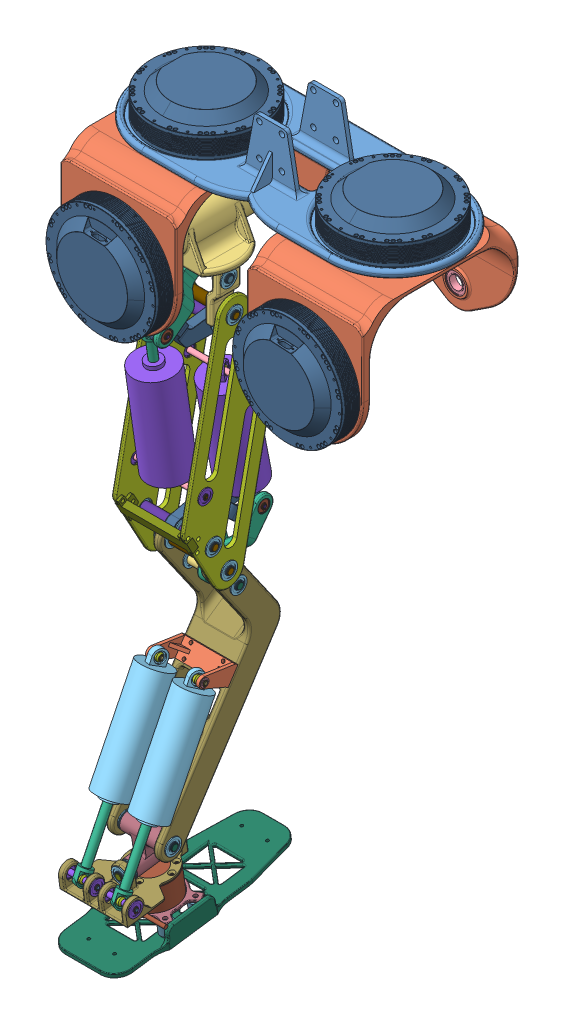
SolidWorks assembly 纯下肢, configuration 默认. Lengths in mm. (continued)
Mates (geometry in assembly coordinates): (continued)
- 重合761: coincident aligned: plane of 法兰轴承10_22_6-53 through (-234.521 -852.1196 -423.0881) normal (-0.219476 0 -0.975618); plane of 10mm轴93mm-1 through (-145 -614.0669 66.1725) normal (0 -0.54068 -0.841228)
- 同心861: concentric aligned: cylinder of 轴承_NSK635-3 through (-168.3887 40.3594 -130.4685) axis (1 0 0) radius 2.5; cylinder of 5mm轴56mm-1 through (-115.4 40.3594 -130.4685) axis (1 0 0) radius 2.5
- 重合771: coincident aligned: plane of 轴承_NSK635-3 through (-173 41.3846 -128.1884) normal (-1 0 0); plane of 5mm轴56mm-1 through (-173 40.3594 -130.4685) normal (-1 0 0)
- 同心871: concentric aligned: cylinder of 轴承_NSK635-9 through (-168.3887 -263.2782 -281.1374) axis (1 0 0) radius 2.5; cylinder of 5mm轴56mm-2 through (-115.4 -263.2782 -281.1374) axis (1 0 0) radius 2.5
- 重合781: coincident aligned: plane of 轴承_NSK635-9 through (-173 -262.4163 -278.7906) normal (-1 0 0); plane of 5mm轴56mm-2 through (-173 -263.2782 -281.1374) normal (-1 0 0)
- 同心881: concentric anti-aligned: cylinder of 法兰轴承5-19-6-1 through (-200.8613 -176.2424 -161.2878) axis (-1 0 0) radius 2.5; cylinder of 5mm轴114.5mm-1 through (-86.15 -176.2424 -161.2878) axis (1 0 0) radius 2.5
- 重合791: coincident aligned: plane of 法兰轴承5-19-6-1 through (-202.25 -180.1137 -162.2944) normal (-1 0 0); plane of 5mm轴114.5mm-1 through (-202.25 -176.2424 -161.2878) normal (-1 0 0)
- 同心891: concentric anti-aligned: cylinder of 法兰轴承5-19-6-2 through (-200.8613 -73.2936 -243.9107) axis (-1 0 0) radius 2.5; cylinder of 5mm轴114.5mm-2 through (-86.15 -73.2936 -243.9107) axis (1 0 0) radius 2.5
- 重合801: coincident aligned: plane of 法兰轴承5-19-6-2 through (-202.25 -75.8193 -240.8089) normal (-1 0 0); plane of 5mm轴114.5mm-2 through (-202.25 -73.2936 -243.9107) normal (-1 0 0)
- 重合811: coincident anti-aligned: cylinder of 法兰轴承5-19-6-9; cylinder of 5mm轴48mm-1 through (-149.3998 -548.3357 168.3569) axis (0.999946 -0.00876 0.00563) radius 2.5
- 重合821: coincident aligned: plane of 法兰轴承5-19-6-9 through (-263.7984 -847.0637 -295.7127) normal (-0.975618 0 0.219476); plane of 5mm轴48mm-1 through (-198.9971 -547.9013 168.0777) normal (-0.999946 0.00876 -0.00563)
- 重合84: coincident anti-aligned: plane of 小腿骨-1 through (-103.25 -625.3653 -108.2044) normal (0 0.544715 0.838621); plane of 脚踝推杆上固定座-1 through (-145 -454.2866 -219.3263) normal (0 -0.544715 -0.838621)
- 同心91: concentric aligned: cylinder of 小腿骨-1 through (-170 -445.9004 -224.7735) axis (0 0.544715 0.838621) radius 2.1; cylinder of 脚踝推杆上固定座-1 through (-170 -445.9004 -224.7735) axis (0 0.544715 0.838621) radius 2.6
- 同心92: concentric aligned: cylinder of 小腿骨-1 through (-120 -462.6728 -213.8792) axis (0 0.544715 0.838621) radius 2.1; cylinder of 脚踝推杆上固定座-1 through (-120 -462.6728 -213.8792) axis (0 0.544715 0.838621) radius 2.6
- 同心902: concentric aligned: cylinder of 脚踝推杆上固定座-1 through (-181.75 -440.6765 -174.5071) axis (-1 0 0) radius 5.5; cylinder of 法兰轴承5_11_5-1 through (-187.3613 -440.6765 -174.5071) axis (-1 0 0) radius 5.5
- 重合832: coincident anti-aligned: plane of 脚踝推杆上固定座-1 through (-186.75 -439.8223 -222.7592) normal (-1 0 0); plane of 法兰轴承5_11_5-1 through (-186.75 -440.6765 -174.5071) normal (1 0 0)
- 同心903: concentric aligned: cylinder of 脚踝推杆上固定座-1 through (-108.25 -440.6765 -174.5071) axis (1 0 0) radius 5.5; cylinder of 法兰轴承5_11_5-2 through (-102.6387 -440.6765 -174.5071) axis (1 0 0) radius 5.5
- 重合833: coincident anti-aligned: plane of 脚踝推杆上固定座-1 through (-103.25 -439.8223 -222.7592) normal (1 0 0); plane of 法兰轴承5_11_5-2 through (-103.25 -440.6765 -174.5071) normal (-1 0 0)
- 同心904: concentric aligned: cylinder of 5mm轴17.25mm-1 through (-100.65 -440.6765 -174.5071) axis (1 0 0) radius 2.5; cylinder of 法兰轴承5_11_5-2 through (-102.6387 -440.6765 -174.5071) axis (1 0 0) radius 2.5
- 重合834: coincident aligned: plane of 5mm轴17.25mm-1 through (-102.25 -440.6765 -174.5071) normal (1 0 0); plane of 法兰轴承5_11_5-2 through (-102.25 -439.866 -177.912) normal (1 0 0)
- 同心905: concentric anti-aligned: cylinder of 5mm轴17.25mm-2 through (-168.9 -440.6765 -174.5071) axis (1 0 0) radius 2.5; cylinder of 法兰轴承5_11_5-1 through (-187.3613 -440.6765 -174.5071) axis (-1 0 0) radius 2.5
- 重合836: coincident aligned: plane of 5mm轴17.25mm-2 through (-187.75 -440.6765 -174.5071) normal (-1 0 0); plane of 法兰轴承5_11_5-1 through (-187.75 -437.2088 -174.0326) normal (-1 0 0)
- 同心906: concentric anti-aligned: cylinder of 5mm轴17.25mm-2 through (-168.9 -440.6765 -174.5071) axis (1 0 0) radius 2.5; cylinder of 脚踝推杆-1/脚踝推杆球头-2 through (-169.5 -440.6765 -174.5071) axis (-1 0 0) radius 2.5
- 重合837: coincident aligned: plane of 5mm轴17.25mm-2 through (-170.5 -440.6765 -174.5071) normal (1 0 0); plane of 脚踝推杆-1/脚踝推杆球头-2 through (-170.5 -440.6765 -174.5071) normal (1 0 0)
- 同心907: concentric anti-aligned: cylinder of 5mm轴48mm-1 through (-149.4 -681.0298 -55.9563) axis (1 0 0) radius 2.5; cylinder of 脚踝推杆-1/脚踝推杆球头-1 through (-169.5 -681.0298 -55.9563) axis (-1 0 0) radius 2.5
- 宽度82: width anti-aligned: plane of 脚踝推杆-1/脚踝推杆伸缩杆-1 through (-178.6027 -550.9935 166.2886) normal (-0.720862 -0.576409 -0.38485); plane of 脚踝推杆-1/脚踝推杆伸缩杆-1 through (-171.3941 -545.2294 170.1371) normal (0.720862 0.576409 0.38485); plane of 脚掌v3.0.1-1 through (-253.5818 -834.6865 -279.9138) normal (0.975618 0 -0.219476); plane of 脚掌v3.0.1-1 through (-225.2889 -834.6865 -286.2786) normal (-0.975618 0 0.219476)
- 同心908: concentric anti-aligned: cylinder of 5mm轴17.25mm-1 through (-100.65 -440.6765 -174.5071) axis (1 0 0) radius 2.5; cylinder of 脚踝推杆-2/脚踝推杆球头-2 through (-109.5 -440.6765 -174.5071) axis (-1 0 0) radius 2.5
- 重合838: coincident aligned: plane of 5mm轴17.25mm-1 through (-119.5 -440.6765 -174.5071) normal (-1 0 0); plane of 脚踝推杆-2/脚踝推杆球头-2 through (-119.5 -440.6765 -174.5071) normal (-1 0 0)
- 同心911: concentric anti-aligned: cylinder of 5mm轴48mm-2 through (-89.4 -681.0298 -55.9563) axis (1 0 0) radius 2.5; cylinder of 脚踝推杆-2/脚踝推杆球头-1 through (-109.5 -681.0298 -55.9563) axis (-1 0 0) radius 2.5
- 宽度83: width anti-aligned: plane of 脚踝推杆-2/脚踝推杆伸缩杆-1 through (-110.5527 -546.7406 169.8196) normal (0.889791 0.379294 0.253788); plane of 脚踝推杆-2/脚踝推杆伸缩杆-1 through (-119.4506 -550.5335 167.2817) normal (-0.889791 -0.379294 -0.253788); plane of 脚掌v3.0.1-1 through (-166.7518 -834.6865 -299.4472) normal (-0.975618 0 0.219476); plane of 脚掌v3.0.1-1 through (-195.0448 -834.6865 -293.0824) normal (0.975618 0 -0.219476)
- 同心912: concentric anti-aligned: cylinder of 5mm轴114.5mm-2 through (-86.15 -73.2936 -243.9107) axis (1 0 0) radius 2.5; cylinder of 膝髋推杆-1/脚踝推杆球头-1 through (-139.5 -73.2936 -243.9107) axis (-1 0 0) radius 2.5
- 宽度84: width aligned: plane of 大腿侧板-2 through (-95.25 -294.2141 -198.324) normal (-1 0 0); plane of 大腿侧板-1 through (-194.75 -294.2141 -198.324) normal (1 0 0); plane of 膝髋推杆-1/脚踝推杆球头-1 through (-149.5 -73.2936 -243.9107) normal (-1 0 0); plane of 膝髋推杆-1/脚踝推杆球头-1 through (-140.5 -73.2936 -243.9107) normal (1 0 0)
- 同心916: concentric anti-aligned: cylinder of 法兰轴承10_22_6-41 through (-186.8613 -335.1743 -226.9991) axis (-1 0 0) radius 5; cylinder of 10mm轴86.5mm-1 through (-99.55 -335.1743 -226.9991) axis (1 0 0) radius 5
- 重合839: coincident aligned: plane of 法兰轴承10_22_6-40 through (-101.75 -340.3354 -230.9505) normal (1 0 0); plane of 10mm轴86.5mm-1 through (-101.75 -335.1743 -226.9991) normal (1 0 0)
- 同心917: concentric anti-aligned: cylinder of 5mm轴56mm-2 through (-115.4 -263.2782 -281.1374) axis (1 0 0) radius 2.5; cylinder of 膝髋推杆-1/脚踝推杆球头-2 through (-139.5 -263.2782 -281.1374) axis (-1 0 0) radius 2.5
- 宽度85: width anti-aligned: plane of 膝髋推杆-1/脚踝推杆球头-2 through (-149.5 -263.2782 -281.1374) normal (-1 0 0); plane of 膝髋推杆-1/脚踝推杆球头-2 through (-140.5 -263.2782 -281.1374) normal (1 0 0); plane of 膝关节U型架-4 through (-165 -286.209 -245.0932) normal (1 0 0); plane of 膝关节U型架-4 through (-125 -254.2552 -269.1547) normal (-1 0 0)
- 同心918: concentric anti-aligned: cylinder of 轴承_NSK635-6 through (-130.6113 -263.2782 -281.1374) axis (-1 0 0) radius 2.5; cylinder of 5mm轴56mm-2 through (-115.4 -263.2782 -281.1374) axis (1 0 0) radius 2.5
- 同心920: concentric anti-aligned: cylinder of 5mm轴114.5mm-1 through (-86.15 -176.2424 -161.2878) axis (1 0 0) radius 2.5; cylinder of 膝髋推杆-2/脚踝推杆球头-1 through (-139.5 -176.2424 -161.2878) axis (-1 0 0) radius 2.5
- 宽度86: width aligned: plane of 大腿侧板-1 through (-194.75 -294.2141 -198.324) normal (1 0 0); plane of 大腿侧板-2 through (-95.25 -294.2141 -198.324) normal (-1 0 0); plane of 膝髋推杆-2/脚踝推杆球头-1 through (-140.5 -176.2424 -161.2878) normal (1 0 0); plane of 膝髋推杆-2/脚踝推杆球头-1 through (-149.5 -176.2424 -161.2878) normal (-1 0 0)
- 同心921: concentric anti-aligned: cylinder of 5mm轴56mm-1 through (-115.4 40.3594 -130.4685) axis (1 0 0) radius 2.5; cylinder of 膝髋推杆-2/脚踝推杆球头-2 through (-139.5 40.3594 -130.4685) axis (-1 0 0) radius 2.5
- 同心923: concentric aligned: cylinder of 5mm轴56mm-1 through (-115.4 40.3594 -130.4685) axis (1 0 0) radius 2.4; cylinder of 轴端挡圈GB894-5-1 through (-173.6 40.3594 -130.4685) axis (1 0 0) radius 2.35
- 重合841: coincident anti-aligned: plane of 轴承_NSK635-3 through (-173 41.3846 -128.1884) normal (-1 0 0); plane of 轴端挡圈GB894-5-1 through (-173 40.2078 -130.2097) normal (1 0 0)
- 同心924: concentric aligned: cylinder of 5mm轴56mm-1 through (-115.4 40.3594 -130.4685) axis (1 0 0) radius 2.4; cylinder of 轴端挡圈GB894-5-2 through (-117 40.3594 -130.4685) axis (1 0 0) radius 2.35
- 重合842: coincident anti-aligned: plane of 轴承_NSK635-4 through (-117 40.8845 -126.5032) normal (1 0 0); plane of 轴端挡圈GB894-5-2 through (-117 40.2078 -130.2097) normal (-1 0 0)
- 同心925: concentric aligned: cylinder of 5mm轴114.5mm-2 through (-86.15 -73.2936 -243.9107) axis (1 0 0) radius 2.4; cylinder of 轴端挡圈GB894-5-3 through (-87.75 -73.2936 -243.9107) axis (1 0 0) radius 2.35
- 重合843: coincident anti-aligned: plane of 法兰轴承5-19-6-6 through (-87.75 -75.8193 -240.8089) normal (1 0 0); plane of 轴端挡圈GB894-5-3 through (-87.75 -72.9942 -243.9295) normal (-1 0 0)
- 同心926: concentric aligned: cylinder of 5mm轴114.5mm-2 through (-86.15 -73.2936 -243.9107) axis (1 0 0) radius 2.4; cylinder of 轴端挡圈GB894-5-4 through (-202.85 -73.2936 -243.9107) axis (1 0 0) radius 2.35
- 重合845: coincident anti-aligned: plane of 法兰轴承5-19-6-2 through (-202.25 -75.8193 -240.8089) normal (-1 0 0); plane of 轴端挡圈GB894-5-4 through (-202.25 -72.9942 -243.9295) normal (1 0 0)
- 重合847: coincident anti-aligned: plane of 法兰轴承5-19-6-1 through (-202.25 -180.1137 -162.2944) normal (-1 0 0); plane of 轴端挡圈GB894-5-5 through (-202.25 -175.9498 -161.2214) normal (1 0 0)
- 同心928: concentric aligned: cylinder of 5mm轴114.5mm-1 through (-86.15 -176.2424 -161.2878) axis (1 0 0) radius 2.4; cylinder of 轴端挡圈GB894-5-5 through (-202.85 -176.2424 -161.2878) axis (1 0 0) radius 2.35
- 重合848: coincident anti-aligned: plane of 法兰轴承5-19-6-5 through (-87.75 -180.1137 -162.2944) normal (1 0 0); plane of 轴端挡圈GB894-5-7 through (-87.75 -175.943 -161.3066) normal (-1 0 0)
- 同心929: concentric aligned: cylinder of 5mm轴114.5mm-1 through (-86.15 -176.2424 -161.2878) axis (1 0 0) radius 2.4; cylinder of 轴端挡圈GB894-5-7 through (-87.75 -176.2424 -161.2878) axis (1 0 0) radius 2.35
- 重合849: coincident anti-aligned: plane of 轴承_NSK635-10 through (-117 -263.237 -277.1376) normal (1 0 0); plane of 轴端挡圈GB894-5-6 through (-117 -262.9788 -281.1562) normal (-1 0 0)
- 同心930: concentric aligned: cylinder of 5mm轴56mm-2 through (-115.4 -263.2782 -281.1374) axis (1 0 0) radius 2.4; cylinder of 轴端挡圈GB894-5-6 through (-117 -263.2782 -281.1374) axis (1 0 0) radius 2.35
- 同心931: concentric anti-aligned: cylinder of 5mm轴56mm-2 through (-115.4 -263.2782 -281.1374) axis (1 0 0) radius 2.4; cylinder of 轴端挡圈GB894-5-8 through (-173 -263.2782 -281.1374) axis (-1 0 0) radius 2.35
- 重合853: coincident anti-aligned: plane of 轴承_NSK635-9 through (-173 -262.4163 -278.7906) normal (-1 0 0); plane of 轴端挡圈GB894-5-8 through (-173 -263.0102 -281.0025) normal (1 0 0)
- 重合854: coincident anti-aligned: plane of 法兰轴承5_11_5-2 through (-102.25 -439.866 -177.912) normal (1 0 0); plane of 轴端挡圈GB894-5-9 through (-102.25 -440.3771 -174.5259) normal (-1 0 0)
- 同心932: concentric aligned: cylinder of 5mm轴17.25mm-1 through (-100.65 -440.6765 -174.5071) axis (1 0 0) radius 2.4; cylinder of 轴端挡圈GB894-5-9 through (-102.25 -440.6765 -174.5071) axis (1 0 0) radius 2.35
- 重合855: coincident anti-aligned: plane of 脚踝推杆-1/脚踝推杆球头-2 through (-170.5 -440.6765 -174.5071) normal (1 0 0); plane of 轴端挡圈GB894-5-10 through (-170.5 -440.3771 -174.5259) normal (-1 0 0)
- 同心933: concentric aligned: cylinder of 5mm轴17.25mm-2 through (-168.9 -440.6765 -174.5071) axis (1 0 0) radius 2.4; cylinder of 轴端挡圈GB894-5-10 through (-170.5 -440.6765 -174.5071) axis (1 0 0) radius 2.35
- 重合856: coincident anti-aligned: plane of 脚踝推杆-2/脚踝推杆球头-2 through (-119.5 -440.6765 -174.5071) normal (-1 0 0); plane of 轴端挡圈GB894-5-11 through (-119.5 -440.5674 -174.7866) normal (1 0 0)
- 同心934: concentric anti-aligned: cylinder of 5mm轴17.25mm-1 through (-100.65 -440.6765 -174.5071) axis (1 0 0) radius 2.4; cylinder of 轴端挡圈GB894-5-11 through (-119.5 -440.6765 -174.5071) axis (-1 0 0) radius 2.35
- 重合857: coincident anti-aligned: plane of 法兰轴承5_11_5-1 through (-187.75 -437.2088 -174.0326) normal (-1 0 0); plane of 轴端挡圈GB894-5-12 through (-187.75 -440.5674 -174.7866) normal (1 0 0)
- 同心935: concentric anti-aligned: cylinder of 5mm轴17.25mm-2 through (-168.9 -440.6765 -174.5071) axis (1 0 0) radius 2.4; cylinder of 轴端挡圈GB894-5-12 through (-187.75 -440.6765 -174.5071) axis (-1 0 0) radius 2.35
- 同心936: concentric aligned: cylinder of 5mm轴48mm-2 through (-89.4 -681.0298 -55.9563) axis (1 0 0) radius 2.4; cylinder of 轴端挡圈GB894-5-13 through (-91 -681.0298 -55.9563) axis (1 0 0) radius 2.35
- 同心937: concentric aligned: cylinder of 5mm轴48mm-1 through (-149.4 -681.0298 -55.9563) axis (1 0 0) radius 2.4; cylinder of 轴端挡圈GB894-5-15 through (-151 -681.0298 -55.9563) axis (1 0 0) radius 2.35
- 重合860: coincident anti-aligned: plane of 法兰轴承5-19-6-9 through (-263.7984 -847.0637 -295.7127) normal (-0.975618 0 0.219476); plane of 轴端挡圈GB894-5-14 through (-198.9945 -547.7923 167.7982) normal (0.999946 -0.00876 0.00563)
- 同心938: concentric anti-aligned: cylinder of 5mm轴48mm-1 through (-149.4 -681.0298 -55.9563) axis (1 0 0) radius 2.4; cylinder of 轴端挡圈GB894-5-14 through (-199 -681.0298 -55.9563) axis (-1 0 0) radius 2.35
- 同心940: concentric aligned: cylinder of 5mm轴48mm-2 through (-89.4 -681.0298 -55.9563) axis (1 0 0) radius 2.4; cylinder of 轴端挡圈GB894-5-17 through (-141.1144 -681.0298 -55.9563) axis (1 0 0) radius 2.35
- 重合862: coincident anti-aligned: plane of 法兰轴承10_22_6-53 through (-234.521 -852.1196 -423.0881) normal (-0.219476 0 -0.975618); plane of 轴端挡圈GB894-10-4 through (-145.3086 -613.5384 65.8328) normal (0 0.54068 0.841228)
- 同心941: concentric aligned: cylinder of 10mm轴93mm-1 through (-145 -677.3369 -81.9957) axis (0 -0.140415 0.990093) radius 4.8; cylinder of 轴端挡圈GB894-10-4 through (-145 -663.829 -177.2427) axis (0 -0.140415 0.990093) radius 4.65
- 重合863: coincident anti-aligned: plane of 法兰轴承10_22_6-45 through (-101.75 -641.693 -129.3475) normal (1 0 0); plane of 轴端挡圈GB894-10-2 through (-101.75 -635.8333 -125.44) normal (-1 0 0)
- 同心942: concentric aligned: cylinder of 10mm轴86.5mm-2 through (-99.55 -636.5319 -125.3961) axis (1 0 0) radius 4.8; cylinder of 轴端挡圈GB894-10-2 through (-101.75 -636.5319 -125.3961) axis (1 0 0) radius 4.65
- 重合864: coincident anti-aligned: plane of 法兰轴承10_22_6-48 through (-188.25 -641.693 -129.3475) normal (-1 0 0); plane of 轴端挡圈GB894-10-1 through (-188.25 -636.2775 -126.0482) normal (1 0 0)
- 同心943: concentric anti-aligned: cylinder of 10mm轴86.5mm-2 through (-99.55 -636.5319 -125.3961) axis (1 0 0) radius 4.8; cylinder of 轴端挡圈GB894-10-1 through (-188.25 -636.5319 -125.3961) axis (-1 0 0) radius 4.65
- 同心944: concentric aligned: cylinder of 10mm轴93mm-1 through (-145 -677.3369 -81.9957) axis (0 -0.140415 0.990093) radius 4.8; cylinder of 轴端挡圈GB894-10-3 through (-145 -677.028 -84.1739) axis (0 -0.140415 0.990093) radius 4.65
- 重合867: coincident anti-aligned: plane of 法兰轴承10_22_6-41 through (-188.25 -340.3354 -230.9505) normal (-1 0 0); plane of 轴端挡圈GB894-10-5 through (-188.25 -334.4757 -227.043) normal (1 0 0)
- 同心945: concentric aligned: cylinder of 10mm轴86.5mm-1 through (-99.55 -335.1743 -226.9991) axis (1 0 0) radius 4.8; cylinder of 轴端挡圈GB894-10-5 through (-189.25 -335.1743 -226.9991) axis (1 0 0) radius 4.65
- 重合868: coincident anti-aligned: plane of 法兰轴承10_22_6-11 through (-202.25 -298.3183 -193.2836) normal (-1 0 0); plane of 轴端挡圈GB894-10-6 through (-202.25 -293.5155 -198.3679) normal (1 0 0)
- 同心946: concentric aligned: cylinder of 10mm轴114.5mm-4 through (-85.55 -294.2141 -198.324) axis (1 0 0) radius 4.8; cylinder of 轴端挡圈GB894-10-6 through (-203.25 -294.2141 -198.324) axis (1 0 0) radius 4.65
- 同心947: concentric aligned: cylinder of 10mm轴114.5mm-3 through (-85.55 -250.296 -174.4241) axis (1 0 0) radius 4.8; cylinder of 轴端挡圈GB894-10-7 through (-203.25 -250.296 -174.4241) axis (1 0 0) radius 4.65
- 重合869: coincident anti-aligned: plane of 法兰轴承10_22_6-12 through (-202.25 -254.4003 -169.3838) normal (-1 0 0); plane of 轴端挡圈GB894-10-7 through (-202.25 -249.5974 -174.468) normal (1 0 0)
- 重合870: coincident anti-aligned: plane of 法兰轴承10_22_6-13 through (-202.25 -2.3445 -225.7592) normal (-1 0 0); plane of 轴端挡圈GB894-10-9 through (-202.25 2.4583 -230.8435) normal (1 0 0)
- 同心948: concentric aligned: cylinder of 10mm轴114.5mm-2 through (-85.55 1.7597 -230.7996) axis (1 0 0) radius 4.8; cylinder of 轴端挡圈GB894-10-9 through (-203.25 1.7597 -230.7996) axis (1 0 0) radius 4.65
- 重合871: coincident anti-aligned: plane of 法兰轴承10_22_6-14 through (-202.25 41.5735 -201.8593) normal (-1 0 0); plane of 轴端挡圈GB894-10-8 through (-202.25 46.3764 -206.9436) normal (1 0 0)
- 同心949: concentric aligned: cylinder of 10mm轴114.5mm-1 through (-85.55 45.6778 -206.8997) axis (1 0 0) radius 4.8; cylinder of 轴端挡圈GB894-10-8 through (-203.25 45.6778 -206.8997) axis (1 0 0) radius 4.65
- 重合872: coincident anti-aligned: plane of 法兰轴承10_22_6-4 through (-198.25 89.2264 -199.651) normal (-1 0 0); plane of 轴端挡圈GB894-10-10 through (-198.25 96.1025 -201.7172) normal (1 0 0)
- 同心950: concentric aligned: cylinder of 10mm轴106.5mm-1 through (-89.55 95.4038 -201.6733) axis (1 0 0) radius 4.8; cylinder of 轴端挡圈GB894-10-10 through (-199.25 95.4038 -201.6733) axis (1 0 0) radius 4.65
- 重合873: coincident anti-aligned: plane of 法兰轴承10_22_6-8 through (-91.75 89.2264 -199.651) normal (1 0 0); plane of 轴端挡圈GB894-10-11 through (-91.75 95.6583 -202.3254) normal (-1 0 0)
- 同心951: concentric anti-aligned: cylinder of 10mm轴106.5mm-1 through (-89.55 95.4038 -201.6733) axis (1 0 0) radius 4.8; cylinder of 轴端挡圈GB894-10-11 through (-90.75 95.4038 -201.6733) axis (-1 0 0) radius 4.65
- 重合874: coincident anti-aligned: plane of 法兰轴承10_22_6-22 through (-87.75 41.5735 -201.8593) normal (1 0 0); plane of 轴端挡圈GB894-10-12 through (-87.75 45.9322 -207.5518) normal (-1 0 0)
- 同心952: concentric anti-aligned: cylinder of 10mm轴114.5mm-1 through (-85.55 45.6778 -206.8997) axis (1 0 0) radius 4.8; cylinder of 轴端挡圈GB894-10-12 through (-86.75 45.6778 -206.8997) axis (-1 0 0) radius 4.65
- 重合875: coincident anti-aligned: plane of 法兰轴承10_22_6-21 through (-87.75 -2.3445 -225.7592) normal (1 0 0); plane of 轴端挡圈GB894-10-13 through (-87.75 2.0141 -231.4517) normal (-1 0 0)
- 同心953: concentric anti-aligned: cylinder of 10mm轴114.5mm-2 through (-85.55 1.7597 -230.7996) axis (1 0 0) radius 4.8; cylinder of 轴端挡圈GB894-10-13 through (-86.75 1.7597 -230.7996) axis (-1 0 0) radius 4.65
- 重合876: coincident anti-aligned: plane of 法兰轴承10_22_6-20 through (-87.75 -254.4003 -169.3838) normal (1 0 0); plane of 轴端挡圈GB894-10-14 through (-87.75 -250.0416 -175.0762) normal (-1 0 0)
- 重合877: coincident anti-aligned: plane of 法兰轴承10_22_6-19 through (-87.75 -298.3183 -193.2836) normal (1 0 0); plane of 轴端挡圈GB894-10-16 through (-87.75 -293.9596 -198.9761) normal (-1 0 0)
- 重合878: coincident anti-aligned: plane of 法兰轴承10_22_6-40 through (-101.75 -340.3354 -230.9505) normal (1 0 0); plane of 轴端挡圈GB894-10-15 through (-101.75 -334.9198 -227.6512) normal (-1 0 0)
- 同心954: concentric anti-aligned: cylinder of 10mm轴86.5mm-1 through (-99.55 -335.1743 -226.9991) axis (1 0 0) radius 4.8; cylinder of 轴端挡圈GB894-10-15 through (-100.75 -335.1743 -226.9991) axis (-1 0 0) radius 4.65
- 同心955: concentric anti-aligned: cylinder of 10mm轴114.5mm-4 through (-85.55 -294.2141 -198.324) axis (1 0 0) radius 4.8; cylinder of 轴端挡圈GB894-10-16 through (-86.75 -294.2141 -198.324) axis (-1 0 0) radius 4.65
- 同心956: concentric anti-aligned: cylinder of 10mm轴114.5mm-3 through (-85.55 -250.296 -174.4241) axis (1 0 0) radius 4.8; cylinder of 轴端挡圈GB894-10-14 through (-86.75 -250.296 -174.4241) axis (-1 0 0) radius 4.65
- 平行12: parallel anti-aligned: plane of 腰部固定座v3.0.3-1 through (-145 285.9038 -219.3997) normal (0 1 0); plane of 脚掌v3.0.1-1 through (-204.4605 -871.6865 -264.3144) normal (0 -1 0)
- 同心966: concentric anti-aligned: cylinder of 10mm轴93mm-1 through (-145 -677.3369 -81.9957) axis (0 -0.140415 0.990093) radius 5; cylinder of 脚踝-1/法兰轴承10_22_6-2 through (-145 -675.3976 -95.6702) axis (0 0.140415 -0.990093) radius 5
- 同心967: concentric anti-aligned: cylinder of 脚踝交叉转轴套筒-1 through (-145 -674.8515 -99.5204) axis (0 0.140415 -0.990093) radius 13; cylinder of 10mm轴93mm-1 through (-145 -677.3369 -81.9957) axis (0 -0.140415 0.990093) radius 5
- 宽度92: width anti-aligned: plane of 脚踝交叉转轴套筒-1 through (-145 -674.8515 -99.5204) normal (0 -0.140415 0.990093); plane of 脚踝-1/脚踝上支承板-1 through (-145 -666.1458 -160.9061) normal (0 0.140415 -0.990093); plane of 脚踝交叉转轴套筒-1 through (-130 -649.3286 -172.6612) normal (0 0.140415 -0.990093); plane of 脚踝-1/脚踝上支承板-1 through (-130 -661.966 -83.5529) normal (0 -0.140415 0.990093)
- 重合893: coincident aligned: plane of 10mm轴93mm-1 through (-145 -663.9694 -176.2526) normal (0 0.140415 -0.990093); plane of 脚踝-1/法兰轴承10_22_6-4 through (-139.5584 -667.4893 -176.7518) normal (0 0.140415 -0.990093)
- 重合894: coincident anti-aligned: plane of 轴端挡圈GB894-10-4 through (-145.3086 -663.3473 -176.1643) normal (0 -0.140415 0.990093); plane of 脚踝-1/法兰轴承10_22_6-4 through (-139.5584 -667.4893 -176.7518) normal (0 0.140415 -0.990093)
- 重合895: coincident anti-aligned: plane of 轴端挡圈GB894-10-3 through (-145.5212 -676.5654 -84.1083) normal (0 0.140415 -0.990093); plane of 脚踝-1/法兰轴承10_22_6-1 through (-151.5 -677.028 -84.1739) normal (0 -0.140415 0.990093)
- 同心968: concentric aligned: cylinder of 5mm轴48mm-2 through (-89.4 -681.0298 -55.9563) axis (1 0 0) radius 2.5; cylinder of 脚踝-1/法兰轴承5-19-6-4 through (-92.3887 -681.0298 -55.9563) axis (1 0 0) radius 2.5
- 同心969: concentric aligned: cylinder of 5mm轴48mm-1 through (-149.4 -681.0298 -55.9563) axis (1 0 0) radius 2.5; cylinder of 脚踝-1/法兰轴承5-19-6-3 through (-152.3887 -681.0298 -55.9563) axis (1 0 0) radius 2.5
- 重合896: coincident aligned: plane of 5mm轴48mm-2 through (-139 -681.0298 -55.9563) normal (-1 0 0); plane of 脚踝-1/法兰轴承5-19-6-2 through (-139 -681.0298 -59.9563) normal (-1 0 0)
- 重合897: coincident aligned: plane of 5mm轴48mm-1 through (-199 -681.0298 -55.9563) normal (-1 0 0); plane of 脚踝-1/法兰轴承5-19-6-1 through (-199 -681.0298 -59.9563) normal (-1 0 0)
- 重合898: coincident anti-aligned: plane of 轴端挡圈GB894-5-14 through (-199 -680.9208 -56.2358) normal (1 0 0); plane of 脚踝-1/法兰轴承5-19-6-1 through (-199 -681.0298 -59.9563) normal (-1 0 0)
- 重合899: coincident anti-aligned: plane of 轴端挡圈GB894-5-15 through (-151 -680.7304 -55.9752) normal (-1 0 0); plane of 脚踝-1/法兰轴承5-19-6-3 through (-151 -684.1923 -53.5071) normal (1 0 0)
- 重合900: coincident anti-aligned: plane of 脚踝-1/法兰轴承5-19-6-4 through (-91 -677.1146 -56.7756) normal (1 0 0); plane of 轴端挡圈GB894-5-13 through (-91 -680.7304 -55.9752) normal (-1 0 0)
- 宽度93: width anti-aligned: plane of 脚踝推杆-2/脚踝推杆球头-1 through (-119.5 -681.0298 -55.9563) normal (-1 0 0); plane of 脚踝-1/脚踝上支承板-1 through (-110.5 -681.0298 -55.9563) normal (1 0 0); plane of 脚踝推杆-2/脚踝推杆球头-1 through (-129.5 -688.1567 -112.5297) normal (1 0 0); plane of 脚踝-1/脚踝上支承板-1 through (-100.5 -688.1567 -112.5297) normal (-1 0 0)
- 宽度94: width anti-aligned: plane of 脚踝-1/脚踝上支承板-1 through (-160.5 -688.1567 -112.5297) normal (-1 0 0); plane of 脚踝推杆-1/脚踝推杆球头-1 through (-189.5 -688.1567 -112.5297) normal (1 0 0); plane of 脚踝-1/脚踝上支承板-1 through (-170.5 -681.0298 -55.9563) normal (1 0 0); plane of 脚踝推杆-1/脚踝推杆球头-1 through (-179.5 -681.0298 -55.9563) normal (-1 0 0)
- 同心973: concentric anti-aligned: cylinder of 法兰轴承10_22_6-33 through (-152.3613 -335.1743 -226.9991) axis (-1 0 0) radius 5; cylinder of 10mm轴86.5mm-1 through (-99.55 -335.1743 -226.9991) axis (1 0 0) radius 5
- 同心974: concentric anti-aligned: cylinder of 法兰轴承10_22_6-43 through (-186.8613 -294.2141 -198.324) axis (-1 0 0) radius 5; cylinder of 10mm轴114.5mm-4 through (-85.55 -294.2141 -198.324) axis (1 0 0) radius 5
- 平行14: parallel anti-aligned: plane of 大腿侧板-1 through (-200.75 -294.2141 -198.324) normal (-1 0 0)
- 重合903: coincident anti-aligned: plane of 大腿侧板-1 through (-190.75 -8.6376 -253.5349) normal (0 0.477998 -0.878361); plane of 大腿侧板柱-5 through (-200.75 -8.6376 -253.5349) normal (0 -0.477998 0.878361)
- 重合904: coincident aligned: plane of 大腿侧板-1 through (-200.75 -294.2141 -198.324) normal (-1 0 0); plane of 大腿侧板柱-5 through (-200.75 -15.0312 -262.7067) normal (-1 0 0)
- 重合905: coincident anti-aligned: plane of 大腿侧板-1 through (-190.75 -3.8576 -262.3185) normal (0 -0.878361 -0.477998); plane of 大腿侧板柱-5 through (-200.75 -3.8576 -262.3185) normal (0 0.878361 0.477998)
- 重合906: coincident anti-aligned: plane of 大腿侧板-1 through (-190.75 -244.6787 -142.9051) normal (0 0.878361 0.477998); plane of 大腿侧板柱-6 through (-89.25 -244.6787 -142.9051) normal (0 -0.878361 -0.477998)
- 重合907: coincident aligned: plane of 大腿侧板-1 through (-200.75 -294.2141 -198.324) normal (-1 0 0); plane of 大腿侧板柱-6 through (-200.75 -233.5051 -142.517) normal (-1 0 0)
- 重合908: coincident anti-aligned: plane of 大腿侧板-1 through (-190.75 -222.3315 -142.1288) normal (0 -0.477998 0.878361); plane of 大腿侧板柱-6 through (-89.25 -222.3315 -142.1288) normal (0 0.477998 -0.878361)
- 同心975: concentric aligned: cylinder of 膝关节U型架后侧-3 through (-183.3627 1.7597 -230.7996) axis (1 0 0) radius 11; cylinder of 10mm轴114.5mm-2 through (-85.55 1.7597 -230.7996) axis (1 0 0) radius 5
- 宽度97: width anti-aligned: plane of 膝关节U型架-3 through (-165 52.9562 -171.2892) normal (1 0 0); plane of 膝关节U型架-3 through (-125 28.492 -139.6426) normal (-1 0 0); plane of 膝关节U型架后侧-3 through (-134 38.5074 -139.5971) normal (-1 0 0); plane of 膝关节U型架后侧-3 through (-156 17.7813 -153.5766) normal (1 0 0)
- 同心976: concentric aligned: cylinder of 膝关节U型架后侧-3 through (-164 40.3594 -130.4685) axis (1 0 0) radius 7.5; cylinder of 5mm轴56mm-1 through (-115.4 40.3594 -130.4685) axis (1 0 0) radius 2.5
- 宽度98: width anti-aligned: plane of 膝关节U型架后侧-3 through (-134 38.5074 -139.5971) normal (-1 0 0); plane of 膝关节U型架后侧-3 through (-156 17.7813 -153.5766) normal (1 0 0); plane of 膝髋推杆-2/脚踝推杆球头-2 through (-140.5 40.3594 -130.4685) normal (1 0 0); plane of 膝髋推杆-2/脚踝推杆球头-2 through (-149.5 40.3594 -130.4685) normal (-1 0 0)
- 同心977: concentric anti-aligned: cylinder of 10mm轴114.5mm-2 through (-85.55 1.7597 -230.7996) axis (1 0 0) radius 5; cylinder of 10mm轴套42.5mm-1 through (-93.75 1.7597 -230.7996) axis (-1 0 0) radius 5
- 同心978: concentric anti-aligned: cylinder of 10mm轴114.5mm-2 through (-85.55 1.7597 -230.7996) axis (1 0 0) radius 5; cylinder of 10mm轴套42.5mm-2 through (-153.75 1.7597 -230.7996) axis (-1 0 0) radius 5
- 重合910: coincident anti-aligned: plane of 法兰轴承10_22_6-28 through (-153.75 -2.0906 -225.5626) normal (-1 0 0); plane of 10mm轴套42.5mm-2 through (-153.75 1.7597 -230.7996) normal (1 0 0)
- 同心979: concentric anti-aligned: cylinder of 10mm轴114.5mm-3 through (-85.55 -250.296 -174.4241) axis (1 0 0) radius 5; cylinder of 10mm轴套42.5mm-3 through (-93.75 -250.296 -174.4241) axis (-1 0 0) radius 7.5
- 同心980: concentric anti-aligned: cylinder of 10mm轴114.5mm-3 through (-85.55 -250.296 -174.4241) axis (1 0 0) radius 5; cylinder of 10mm轴套42.5mm-4 through (-153.75 -250.296 -174.4241) axis (-1 0 0) radius 7.5
- 同心981: concentric anti-aligned: cylinder of 10mm轴114.5mm-1 through (-85.55 45.6778 -206.8997) axis (1 0 0) radius 5; cylinder of 10mm轴套60.5mm-1 through (-115.75 45.6778 -206.8997) axis (-1 0 0) radius 7.5
- 重合913: coincident anti-aligned: plane of 法兰轴承10_22_6-6 through (-115.75 43.9524 -200.6328) normal (-1 0 0); plane of 10mm轴套60.5mm-1 through (-115.75 45.6778 -206.8997) normal (1 0 0)
- 同心982: concentric anti-aligned: cylinder of 10mm轴114.5mm-4 through (-85.55 -294.2141 -198.324) axis (1 0 0) radius 5; cylinder of 10mm轴套60.5mm-2 through (-114.75 -294.2141 -198.324) axis (-1 0 0) radius 7.5
- 重合914: coincident anti-aligned: plane of 法兰轴承10_22_6-39 through (-114.75 -292.1714 -192.1533) normal (-1 0 0); plane of 10mm轴套60.5mm-2 through (-114.75 -294.2141 -198.324) normal (1 0 0)
- 同心983: concentric anti-aligned: cylinder of 10mm轴106.5mm-1 through (-89.55 95.4038 -201.6733) axis (1 0 0) radius 5; cylinder of 10mm轴套30.5mm-1 through (-153.75 95.4038 -201.6733) axis (-1 0 0) radius 7.5
- 重合915: coincident anti-aligned: plane of 法兰轴承10_22_6-9 through (-153.75 93.1003 -207.7514) normal (-1 0 0); plane of 10mm轴套30.5mm-1 through (-153.75 95.4038 -201.6733) normal (1 0 0)
- 重合916: coincident anti-aligned: plane of 法兰轴承10_22_6-10 through (-136.25 89.101 -203.2619) normal (1 0 0); plane of 10mm轴套30.5mm-2 through (-136.25 95.4038 -201.6733) normal (-1 0 0)
- 同心984: concentric anti-aligned: cylinder of 10mm轴106.5mm-1 through (-89.55 95.4038 -201.6733) axis (1 0 0) radius 5; cylinder of 10mm轴套30.5mm-2 through (-105.75 95.4038 -201.6733) axis (-1 0 0) radius 7.5
- 同心985: concentric anti-aligned: cylinder of 10mm轴114.5mm-4 through (-85.55 -294.2141 -198.324) axis (1 0 0) radius 5; cylinder of 10mm轴套8mm-1 through (-188.25 -294.2141 -198.324) axis (-1 0 0) radius 7.5
- 同心986: concentric anti-aligned: cylinder of 10mm轴114.5mm-4 through (-85.55 -294.2141 -198.324) axis (1 0 0) radius 5; cylinder of 10mm轴套8mm-2 through (-93.75 -294.2141 -198.324) axis (-1 0 0) radius 7.5
- 同心987: concentric anti-aligned: cylinder of 10mm轴114.5mm-1 through (-85.55 45.6778 -206.8997) axis (1 0 0) radius 5; cylinder of 10mm轴套8mm-3 through (-188.25 45.6778 -206.8997) axis (-1 0 0) radius 7.5
- 重合920: coincident anti-aligned: plane of 法兰轴承10_22_6-3 through (-188.25 43.3721 -212.977) normal (-1 0 0); plane of 10mm轴套8mm-3 through (-188.25 45.6778 -206.8997) normal (1 0 0)
- 重合921: coincident anti-aligned: plane of 法兰轴承10_22_6-22 through (-93.75 42.5206 -203.0225) normal (-1 0 0); plane of 10mm轴套8mm-4 through (-93.75 45.6778 -206.8997) normal (1 0 0)
- 同心988: concentric anti-aligned: cylinder of 10mm轴114.5mm-1 through (-85.55 45.6778 -206.8997) axis (1 0 0) radius 5; cylinder of 10mm轴套8mm-4 through (-93.75 45.6778 -206.8997) axis (-1 0 0) radius 7.5
- 同心989: concentric anti-aligned: cylinder of 10mm轴86.5mm-1 through (-99.55 -335.1743 -226.9991) axis (1 0 0) radius 5; cylinder of 10mm轴套21.5mm-1 through (-153.75 -335.1743 -226.9991) axis (-1 0 0) radius 7.5
- 重合922: coincident anti-aligned: plane of 法兰轴承10_22_6-33 through (-153.75 -336.6835 -233.3215) normal (-1 0 0); plane of 10mm轴套21.5mm-1 through (-153.75 -335.1743 -226.9991) normal (1 0 0)
- 同心990: concentric anti-aligned: cylinder of 10mm轴86.5mm-1 through (-99.55 -335.1743 -226.9991) axis (1 0 0) radius 5; cylinder of 10mm轴套21.5mm-2 through (-114.75 -335.1743 -226.9991) axis (-1 0 0) radius 7.5
- 重合923: coincident anti-aligned: plane of 法兰轴承10_22_6-34 through (-136.25 -341.2385 -229.3391) normal (1 0 0); plane of 10mm轴套21.5mm-2 through (-136.25 -335.1743 -226.9991) normal (-1 0 0)
- 同心992: concentric anti-aligned: cylinder of 5mm轴114.5mm-2 through (-86.15 -73.2936 -243.9107) axis (1 0 0) radius 2.5; cylinder of 5mm轴套46.75mm-1 through (-93.75 -73.2936 -243.9107) axis (-1 0 0) radius 4
- 同心993: concentric anti-aligned: cylinder of 5mm轴114.5mm-2 through (-86.15 -73.2936 -243.9107) axis (1 0 0) radius 2.5; cylinder of 5mm轴套46.75mm-4 through (-149.5 -73.2936 -243.9107) axis (-1 0 0) radius 4
- 同心994: concentric anti-aligned: cylinder of 5mm轴114.5mm-1 through (-86.15 -176.2424 -161.2878) axis (1 0 0) radius 2.5; cylinder of 5mm轴套46.75mm-2 through (-93.75 -176.2424 -161.2878) axis (-1 0 0) radius 4
- 重合926: coincident anti-aligned: plane of 法兰轴承5-19-6-7 through (-96.75 -124.5949 -289.3868) normal (-1 0 0); plane of 5mm轴套46.75mm-2 through (-93.75 -162.6226 -117.7933) normal (1 0 0)
- 同心995: concentric anti-aligned: cylinder of 5mm轴114.5mm-1 through (-86.15 -176.2424 -161.2878) axis (1 0 0) radius 2.5; cylinder of 5mm轴套46.75mm-3 through (-149.5 -176.2424 -161.2878) axis (-1 0 0) radius 4
- 重合928: coincident anti-aligned: plane of 法兰轴承10_22_6-57 through (-139.7194 -662.1825 -161.8591) normal (0 0.140415 -0.990093); plane of 10mm垫片1mm-4 through (-145 -665.9352 -162.3913) normal (0 -0.140415 0.990093)
- 同心996: concentric anti-aligned: cylinder of 10mm轴93mm-1 through (-145 -677.3369 -81.9957) axis (0 -0.140415 0.990093) radius 5; cylinder of 10mm垫片1mm-4 through (-145 -665.9352 -162.3913) axis (0 0.140415 -0.990093) radius 7.5
- 重合929: coincident anti-aligned: plane of 脚踝-1/法兰轴承10_22_6-2 through (-142.0516 -680.938 -97.8585) normal (0 0.140415 -0.990093); plane of 10mm垫片1mm-1 through (-145 -675.2026 -97.0451) normal (0 -0.140415 0.990093)
- 同心997: concentric anti-aligned: cylinder of 10mm轴93mm-1 through (-145 -677.3369 -81.9957) axis (0 -0.140415 0.990093) radius 5; cylinder of 10mm垫片1mm-1 through (-145 -675.2026 -97.0451) axis (0 0.140415 -0.990093) radius 7.5
- 重合930: coincident anti-aligned: plane of 法兰轴承10_22_6-46 through (-114.75 -634.4893 -119.2254) normal (-1 0 0); plane of 10mm垫片1mm-3 through (-114.75 -636.5319 -125.3961) normal (1 0 0)
- 同心998: concentric anti-aligned: cylinder of 10mm轴86.5mm-2 through (-99.55 -636.5319 -125.3961) axis (1 0 0) radius 5; cylinder of 10mm垫片1mm-3 through (-114.75 -636.5319 -125.3961) axis (-1 0 0) radius 7.5
- 重合931: coincident anti-aligned: plane of 法兰轴承10_22_6-50 through (-174.25 -641.8819 -129.0877) normal (-1 0 0); plane of 10mm垫片1mm-2 through (-174.25 -636.5319 -125.3961) normal (1 0 0)
- 同心999: concentric anti-aligned: cylinder of 10mm轴86.5mm-2 through (-99.55 -636.5319 -125.3961) axis (1 0 0) radius 5; cylinder of 10mm垫片1mm-2 through (-174.25 -636.5319 -125.3961) axis (-1 0 0) radius 7.5
- 重合932: coincident anti-aligned: plane of 轴承_NSK635-10 through (-123 -263.2525 -278.6375) normal (-1 0 0); plane of 5mm轴套3mm-1 through (-123 -263.2782 -281.1374) normal (1 0 0)
- 同心1000: concentric anti-aligned: cylinder of 5mm轴56mm-2 through (-115.4 -263.2782 -281.1374) axis (1 0 0) radius 2.5; cylinder of 5mm轴套3mm-1 through (-123 -263.2782 -281.1374) axis (-1 0 0) radius 4
- 重合933: coincident anti-aligned: plane of 轴承_NSK635-9 through (-167 -261.8992 -277.3826) normal (1 0 0); plane of 5mm轴套3mm-2 through (-167 -263.2782 -281.1374) normal (-1 0 0)
- 同心1001: concentric aligned: cylinder of 5mm轴56mm-2 through (-115.4 -263.2782 -281.1374) axis (1 0 0) radius 2.5; cylinder of 5mm轴套3mm-2 through (-167 -263.2782 -281.1374) axis (1 0 0) radius 4
- 重合934: coincident anti-aligned: plane of 轴承_NSK635-4 through (-123 40.6876 -127.9902) normal (-1 0 0); plane of 5mm轴套3mm-3 through (-123 40.3594 -130.4685) normal (1 0 0)
- 同心1002: concentric anti-aligned: cylinder of 5mm轴56mm-1 through (-115.4 40.3594 -130.4685) axis (1 0 0) radius 2.5; cylinder of 5mm轴套3mm-3 through (-123 40.3594 -130.4685) axis (-1 0 0) radius 4
- 重合935: coincident anti-aligned: plane of 轴承_NSK635-2 through (-164 38.9432 -134.2094) normal (-1 0 0); plane of 5mm轴套3mm-4 through (-164 40.3594 -130.4685) normal (1 0 0)
- 同心1003: concentric anti-aligned: cylinder of 5mm轴56mm-1 through (-115.4 40.3594 -130.4685) axis (1 0 0) radius 2.5; cylinder of 5mm轴套3mm-4 through (-164 40.3594 -130.4685) axis (-1 0 0) radius 4
- 重合936: coincident anti-aligned: plane of 膝髋推杆-1/脚踝推杆球头-2 through (-140.5 -263.2782 -281.1374) normal (1 0 0); plane of 5mm轴套8.5mm-1 through (-140.5 -263.2782 -281.1374) normal (-1 0 0)
- 同心1004: concentric aligned: cylinder of 5mm轴56mm-2 through (-115.4 -263.2782 -281.1374) axis (1 0 0) radius 2.5; cylinder of 5mm轴套8.5mm-1 through (-140.5 -263.2782 -281.1374) axis (1 0 0) radius 4
- 重合937: coincident anti-aligned: plane of 轴承_NSK635-5 through (-158 -263.0327 -283.6253) normal (1 0 0); plane of 5mm轴套8.5mm-2 through (-158 -263.2782 -281.1374) normal (-1 0 0)
- 同心1005: concentric aligned: cylinder of 5mm轴56mm-2 through (-115.4 -263.2782 -281.1374) axis (1 0 0) radius 2.5; cylinder of 5mm轴套8.5mm-2 through (-158 -263.2782 -281.1374) axis (1 0 0) radius 4
- 同心1006: concentric aligned: cylinder of 5mm轴56mm-1 through (-115.4 40.3594 -130.4685) axis (1 0 0) radius 2.5; cylinder of 5mm轴套8.5mm-4 through (-140.5 40.3594 -130.4685) axis (1 0 0) radius 4
- 重合938: coincident anti-aligned: plane of 轴承_NSK635-2 through (-158 39.4743 -132.8066) normal (1 0 0); plane of 5mm轴套8.5mm-3 through (-158 40.3594 -130.4685) normal (-1 0 0)
- 同心1008: concentric aligned: cylinder of 5mm轴56mm-1 through (-115.4 40.3594 -130.4685) axis (1 0 0) radius 2.5; cylinder of 5mm轴套8.5mm-3 through (-158 40.3594 -130.4685) axis (1 0 0) radius 4
- 重合939: coincident anti-aligned: plane of 膝髋推杆-2/脚踝推杆球头-2 through (-140.5 40.3594 -130.4685) normal (1 0 0); plane of 5mm轴套8.5mm-4 through (-140.5 40.3594 -130.4685) normal (-1 0 0)
- 同心1009: concentric aligned: cylinder of 5mm轴48mm-1 through (-149.4 -681.0298 -55.9563) axis (1 0 0) radius 2.5; cylinder of 5mm轴套13.5mm-2 through (-170.5 -681.0298 -55.9563) axis (1 0 0) radius 4
- 同心1010: concentric aligned: cylinder of 5mm轴48mm-2 through (-89.4 -681.0298 -55.9563) axis (1 0 0) radius 2.5; cylinder of 5mm轴套13.5mm-3 through (-133 -681.0298 -55.9563) axis (1 0 0) radius 4
- 同心1011: concentric aligned: cylinder of 5mm轴48mm-2 through (-89.4 -681.0298 -55.9563) axis (1 0 0) radius 2.5; cylinder of 5mm轴套13.5mm-4 through (-110.5 -681.0298 -55.9563) axis (1 0 0) radius 4
- 同心1012: concentric anti-aligned: cylinder of 5mm轴48mm-1 through (-149.4 -681.0298 -55.9563) axis (1 0 0) radius 2.5; cylinder of 5mm轴套13.5mm-1 through (-181.9256 -681.0298 -55.9563) axis (-1 0 0) radius 4
- 平行16: parallel anti-aligned: plane of 脚踝推杆-1/脚踝推杆球头-1 through (-179.5 -681.0298 -55.9563) normal (-1 0 0); plane of 5mm轴套13.5mm-1 through (-181.9256 -681.0298 -55.9563) normal (1 0 0)
- 重合941: coincident anti-aligned: plane of 脚踝推杆-1/脚踝推杆球头-1 through (-170.5 -681.0298 -55.9563) normal (1 0 0); plane of 5mm轴套13.5mm-2 through (-170.5 -681.0298 -55.9563) normal (-1 0 0)
- 重合943: coincident anti-aligned: plane of 脚踝推杆-2/脚踝推杆球头-1 through (-110.5 -681.0298 -55.9563) normal (1 0 0); plane of 5mm轴套13.5mm-4 through (-110.5 -681.0298 -55.9563) normal (-1 0 0)
- 重合944: coincident anti-aligned: plane of 脚踝-1/法兰轴承5-19-6-2 through (-133 -681.0298 -58.4563) normal (1 0 0); plane of 5mm轴套13.5mm-3 through (-133 -681.0298 -55.9563) normal (-1 0 0)
- 同心1013: concentric anti-aligned: cylinder of 5mm轴17.25mm-1 through (-100.65 -440.6765 -174.5071) axis (1 0 0) radius 2.5; cylinder of 5mm轴套3.25mm-1 through (-107.25 -440.6765 -174.5071) axis (-1 0 0) radius 4
- 重合946: coincident anti-aligned: plane of 法兰轴承5_11_5-2 through (-107.25 -440.0976 -176.9391) normal (-1 0 0); plane of 5mm轴套3.25mm-1 through (-107.25 -440.6765 -174.5071) normal (1 0 0)
- 同心1014: concentric anti-aligned: cylinder of 5mm轴17.25mm-2 through (-168.9 -440.6765 -174.5071) axis (1 0 0) radius 2.5; cylinder of 5mm轴套3.25mm-2 through (-179.5 -440.6765 -174.5071) axis (-1 0 0) radius 4
- 重合947: coincident anti-aligned: plane of 脚踝推杆-1/脚踝推杆球头-2 through (-179.5 -440.6765 -174.5071) normal (-1 0 0); plane of 5mm轴套3.25mm-2 through (-179.5 -440.6765 -174.5071) normal (1 0 0)
- 同心1017: concentric anti-aligned: cylinder of 髋侧摆轴v3.0.5-1 through (-145 150.4038 -315.8997) axis (0 0 -1) radius 10; cylinder of 20mm法兰轴承F63804ZZ-1 through (-145 150.4038 -317.3997) axis (0 0 1) radius 10
- 重合950: coincident aligned: plane of 髋侧摆轴v3.0.5-1 through (-145 159.9038 -327.3997) normal (0 0 -1); plane of 20mm法兰轴承F63804ZZ-1 through (-145 150.4038 -327.3997) normal (0 0 -1)
- 重合961: coincident anti-aligned: plane of 腰部固定座v3.0.3-1 through (-80 279.9038 -219.3997) normal (0 1 0); plane of B1电机模型-4 through (-203.8492 279.9038 -219.0874) normal (0 -1 0)
- 重合962: coincident anti-aligned: plane of 腰部固定座v3.0.3-1 through (80 279.9038 -219.3997) normal (0 1 0); plane of B1电机模型-3 through (86.1508 279.9038 -219.0874) normal (0 -1 0)
- 同心1022: concentric aligned: cone of 腰部固定座v3.0.3-1 through (145 279.9038 -219.3997) axis (0 -1 0); cylinder of B1电机模型-3 through (145 237.7038 -219.3997) axis (0 -1 0) radius 58.85
- 同心1023: concentric anti-aligned: cylinder of 腰部固定座v3.0.3-1 through (-145 285.9038 -219.3997) axis (0 1 0) radius 65; cylinder of B1电机模型-4 through (-145 237.7038 -219.3997) axis (0 -1 0) radius 58.85
- 重合964: coincident anti-aligned: plane of 髋旋转轴v3.0.5-2 through (145 65.4038 -88.3997) normal (0 0 1); plane of B1电机模型-1 through (148.2994 209.1613 -88.3997) normal (0 0 -1)
- 同心1024: concentric anti-aligned: cylinder of B1电机模型-1 through (145 150.4038 -130.5997) axis (0 0 -1) radius 58.85; cylinder of 髋旋转轴v3.0.5-2 through (145 150.4038 -82.3997) axis (0 0 1) radius 65
- 重合966: coincident anti-aligned: plane of 髋旋转轴v3.0.5-2 through (145 270.4038 -219.3997) normal (0 1 0); plane of B1电机模型-3 through (178.9093 270.4038 -244.1819) normal (0 -1 0)
- 重合968: coincident aligned: cylinder of 腰部固定座v3.0.3-1 through (145 285.9038 -219.3997) axis (0 1 0) radius 65; unknown of 髋旋转轴v3.0.5-2
- 同心1025: concentric anti-aligned: cylinder of 髋旋转轴v3.0.5-1 through (-145 150.4038 -82.3997) axis (0 0 1) radius 65; cylinder of B1电机模型-2 through (-145 150.4038 -130.5997) axis (0 0 -1) radius 58.85
- 重合970: coincident anti-aligned: plane of 髋旋转轴v3.0.5-1 through (-145 65.4038 -88.3997) normal (0 0 1); plane of B1电机模型-2 through (-141.7006 209.1613 -88.3997) normal (0 0 -1)
- 重合971: coincident anti-aligned: plane of 髋侧摆轴v3.0.5-1 through (-145 174.9038 -97.8997) normal (0 0 1); plane of B1电机模型-2 through (-122.3452 115.0378 -97.8997) normal (0 0 -1)
- 同心1028: concentric aligned: cylinder of 髋旋转轴v3.0.5-1 through (-145 150.4038 -82.3997) axis (0 0 1) radius 16; cylinder of 20mm法兰轴承F63804ZZ-1 through (-145 150.4038 -317.3997) axis (0 0 1) radius 16
- 重合973: coincident anti-aligned: plane of 法兰轴承5-19-6-2 through (-196.25 -74.8722 -241.9721) normal (1 0 0); plane of 5mm轴套46.75mm-4 through (-196.25 -73.2936 -243.9107) normal (-1 0 0)
- 重合974: coincident anti-aligned: plane of 法兰轴承5-19-6-1 through (-196.25 -178.662 -161.9169) normal (1 0 0); plane of 5mm轴套46.75mm-3 through (-196.25 -176.2424 -161.2878) normal (-1 0 0)
- 重合975: coincident anti-aligned: plane of 法兰轴承10_22_6-27 through (-136.25 7.6315 -228.0118) normal (1 0 0); plane of 10mm轴套42.5mm-1 through (-136.25 1.7597 -230.7996) normal (-1 0 0)
- 重合976: coincident anti-aligned: plane of 法兰轴承10_22_6-29 through (-136.25 -246.2735 -169.3183) normal (1 0 0); plane of 10mm轴套42.5mm-3 through (-136.25 -250.296 -174.4241) normal (-1 0 0)
- 同心1029: concentric aligned: cylinder of 法兰轴承10_22_6-29 through (-137.6387 -250.296 -174.4241) axis (1 0 0) radius 5; cylinder of 10mm轴114.5mm-3 through (-85.55 -250.296 -174.4241) axis (1 0 0) radius 5
- 重合977: coincident anti-aligned: plane of 法兰轴承10_22_6-12 through (-196.25 -253.4531 -170.5469) normal (1 0 0); plane of 10mm轴套42.5mm-4 through (-196.25 -250.296 -174.4241) normal (-1 0 0)
- 重合978: coincident anti-aligned: plane of 法兰轴承10_22_6-19 through (-93.75 -297.3712 -194.4468) normal (-1 0 0); plane of 10mm轴套8mm-2 through (-93.75 -294.2141 -198.324) normal (1 0 0)
- 重合979: coincident anti-aligned: plane of 法兰轴承10_22_6-11 through (-196.25 -297.3712 -194.4468) normal (1 0 0); plane of 10mm轴套8mm-1 through (-196.25 -294.2141 -198.324) normal (-1 0 0)
- 重合980: coincident anti-aligned: plane of 髋旋转轴v3.0.5-1 through (-145 270.4038 -219.3997) normal (0 1 0); plane of B1电机模型-4 through (-111.0907 270.4038 -244.1819) normal (0 -1 0)
- 同心1030: concentric anti-aligned: cylinder of 腰部固定座v3.0.3-1 through (-145 285.9038 -219.3997) axis (0 1 0) radius 65; cylinder of 髋旋转轴v3.0.5-1 through (-145 60.4028 -219.3997) axis (0 -1 0) radius 65
- 重合981: coincident anti-aligned: plane of 法兰轴承5-19-6-6 through (-93.75 -74.8722 -241.9721) normal (-1 0 0); plane of 5mm轴套46.75mm-1 through (-93.75 -73.2936 -243.9107) normal (1 0 0)
- 重合982: coincident anti-aligned: plane of 法兰轴承5-19-6-5 through (-93.75 -178.662 -161.9169) normal (-1 0 0); plane of 5mm轴套46.75mm-2 through (-93.75 -176.2424 -161.2878) normal (1 0 0)
- 重合983: coincident: plane of 腰部固定座v3.0.3-1 through (0 279.9038 -219.3997) normal (1 0 0)
- 同心1032: concentric aligned: cylinder of 20mm法兰轴承F63804ZZ-3 through (145 150.4038 -317.3997) axis (0 0 1) radius 16; cylinder of 髋旋转轴v3.0.5-2 through (145 150.4038 -82.3997) axis (0 0 1) radius 16
- 同心1033: concentric anti-aligned: cylinder of 小腿骨-1 through (-94.25 -335.1743 -226.9991) axis (-1 0 0) radius 11; cylinder of 10mm轴86.5mm-1 through (-99.55 -335.1743 -226.9991) axis (1 0 0) radius 5
- 同心1037: concentric aligned: cylinder of 大腿侧板-1 through (-200.75 -294.2141 -198.324) axis (1 0 0) radius 11; cylinder of 10mm轴114.5mm-4 through (-85.55 -294.2141 -198.324) axis (1 0 0) radius 5
- 同心1038: concentric anti-aligned: cylinder of 法兰轴承10_22_6-12 through (-200.75 -250.296 -174.4241) axis (-1 0 0) radius 12.5; cylinder of 10mm轴114.5mm-3 through (-85.55 -250.296 -174.4241) axis (1 0 0) radius 5
- 同心1039: concentric anti-aligned: cylinder of 大腿侧板-1 through (-200.75 -294.2141 -198.324) axis (1 0 0) radius 11; cylinder of 法兰轴承10_22_6-11 through (-200.8613 -294.2141 -198.324) axis (-1 0 0) radius 11
- 重合993: coincident anti-aligned: plane of 大腿侧板-1 through (-200.75 -294.2141 -198.324) normal (-1 0 0); plane of 法兰轴承10_22_6-11 through (-200.75 -294.2141 -198.324) normal (1 0 0)
- 同心1041: concentric anti-aligned: cylinder of 法兰轴承10_22_6-39 through (-113.3613 -294.2141 -198.324) axis (-1 0 0) radius 5; cylinder of 10mm轴114.5mm-4 through (-85.55 -294.2141 -198.324) axis (1 0 0) radius 5
